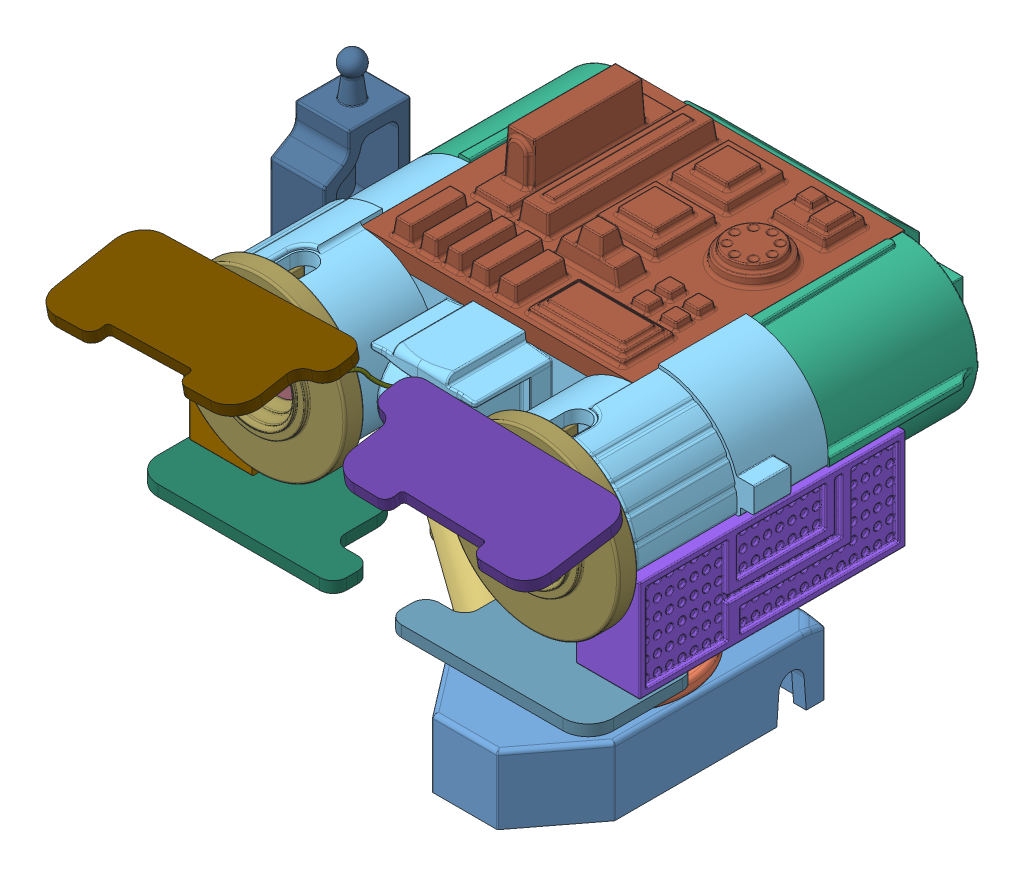
SolidWorks assembly Head, configuration Painted. Lengths in mm.
Overall size (59.38 58.47 64.88).
20 component instances, 18 part files, 63 mates.
Components (placement in the parent):
- Neck Block-1: Neck Block [Default] at origin size (19.8 8.1 32.9)
- Neck Column-1: Neck Column [Default] at (0 8.1 0) size (19.3 30.7 19.3)
- Neck Cylinders-1: Neck Cylinders [Default] at (0 9.78 6.15) size (41.82 28.67 7.85)
- Washer Head Thread-Forming Screw 2.6mm x 6mm-1: Washer Head Thread-Forming Screw 2.6mm x 6mm [Default] at (0 11.65 0) x (-0.707107 0 -0.707107) z (-0.707107 0 0.707107) size (7.8 7.44 7.8)
- Head (Front)-1: Head (Front) [Default] at (0 40.98 0) size (53.5 23.44 24.2)
- Head (Rear)-1: Head (Rear) [Default] at (0 40.98 0) size (51.98 22.63 26)
- Cheese Head Thread-Forming Screw 2.8mm x 8mm-1: Cheese Head Thread-Forming Screw 2.8mm x 8mm [Default] at (0 40.98 3.65) x (0.707107 -0.707107 0) z (0.707107 0.707107 0) size (5.45 9.97 5.45)
- Cheek (Left)-1: Cheek (Left) [Default] at (16.25 40.98 23) size (7.5 12 31.6)
- Cheek (Right)-1: Cheek (Right) [Default] at (-16.25 40.98 23) size (7.5 12 31.6)
- Whip Antenna-1: Whip Antenna [Default] at (-26.586 40.0668 10.4) size (6.56 18.4 10.28)
- Head Detail Plate-1: Head Detail Plate [Default] at (0 47.98 -2.935) size (32.69 7.75 31.87)
- Eye-3: Eye [Default] at (-16.25 40.98 23) size (20.5 20.5 7.96)
- Eye-4: Eye [Default] at (16.25 40.98 23) size (20.5 20.5 7.96)
- Lens-1: Lens [Painted] at (-16.25 40.98 23) size (10.8 10.8 0.8)
- Lens-2: Lens [Painted] at (16.25 40.98 23) size (10.8 10.8 0.8)
- Lower Eyeflap (Left)-1: Lower Eyeflap (Left) [Default] at (3.25 26.4828 29.4) size (23.8 1.32 12.82)
- Lower Eyeflap (Right)-1: Lower Eyeflap (Right) [Default] at (-3.25 26.4828 29.4) size (23.8 1.32 12.82)
- Eyeflap Wire-1: Eyeflap Wire [Default] at (0 46.2834 36.3285) x (1 0 0) z (0 0.173648 0.984808) size (22.36 3.31 16.37)
- Upper Eyeflap (Left)-1: Upper Eyeflap (Left) [Default] at (2.6277 49.0084 30.8173) x (0.99978 -0.019812 0.006846) z (-0.010094 -0.168795 0.985599) size (26.82 1.32 12.82)
- Upper Eyeflap (Right)-1: Upper Eyeflap (Right) [Default] at (-2.6331 49.0082 30.8174) x (0.999778 0.019901 -0.006876) z (0.010139 -0.168839 0.985592) size (26.82 1.32 12.82)
Mates (geometry in assembly coordinates):
- ROTATION LOCK: coincident aligned: plane of Neck Column-1 through (0 8.1 0) normal (0 0 1); plane of assembly through (0 0 0) normal (0 0 1)
- Coincident1: coincident: plane of Neck Block-1 through (0 0 0) normal (0 0 1); plane of assembly through (0 0 0) normal (0 0 1)
- Coincident2: coincident: plane of Neck Block-1 through (0 0 0) normal (0 1 0); plane of assembly through (0 0 0) normal (0 1 0)
- Coincident3: coincident aligned: plane of Neck Block-1 through (0 0 0) normal (1 0 0); plane of assembly through (0 0 0) normal (1 0 0)
- Concentric1: concentric anti-aligned: cylinder of Neck Block-1 through (0 8.1 0) axis (0 -1 0) radius 3; cylinder of Neck Column-1 through (0 5.85 0) axis (0 1 0) radius 2.885
- Coincident4: coincident anti-aligned: plane of Neck Block-1 through (0 8.1 0) normal (0 1 0); plane of Neck Column-1 through (0 8.1 0) normal (0 -1 0)
- Coincident12: coincident anti-aligned: plane of Neck Column-1 through (0 9.78 0) normal (0 1 0); plane of Neck Cylinders-1 through (0 9.78 6.15) normal (0 -1 0)
- Coincident13: coincident aligned: plane of Neck Column-1 through (0 8.1 0) normal (1 0 0); plane of Neck Cylinders-1 through (0 9.78 6.15) normal (1 0 0)
- Coincident14: coincident anti-aligned: plane of Neck Column-1 through (0 8.1 3.825) normal (0 0 1); plane of Neck Cylinders-1 through (0 10.78 3.825) normal (0 0 -1)
- Coincident6: coincident anti-aligned: plane of Head (Front)-1 through (0 40.0668 10.4) normal (0 1 0); plane of Whip Antenna-1 through (-23.306 40.0668 0.12) normal (0 -1 0)
- Coincident7: coincident anti-aligned: plane of Head (Front)-1 through (0 40.98 10.4) normal (0 0 -1); plane of Whip Antenna-1 through (-23.306 40.0668 10.4) normal (0 0 1)
- Coincident8: coincident anti-aligned: plane of Head (Front)-1 through (-23.306 40.98 10.4) normal (-1 0 0); plane of Whip Antenna-1 through (-23.306 40.0668 10.4) normal (1 0 0)
- Coincident16: coincident anti-aligned: plane of Head (Front)-1 through (-10.5931 47.98 -36.225) normal (0 1 0); plane of Head Detail Plate-1 through (0 47.98 -2.935) normal (0 -1 0)
- Coincident17: coincident anti-aligned: plane of Head (Front)-1 through (-16.25 40.98 13) normal (0 0 -1); plane of Head Detail Plate-1 through (-16.345 50.01 13) normal (0 0 1)
- Width1: width aligned: plane of Head Detail Plate-1 through (-16.345 50.01 13) normal (-1 0 0); plane of Head Detail Plate-1 through (16.345 50.01 13) normal (1 0 0); plane of Head (Front)-1 through (16.4 49.98 45.8609) normal (-1 0 0); plane of Head (Front)-1 through (-16.4 49.9787 37.0587) normal (1 0 0)
- Concentric9: concentric aligned: cylinder of Neck Column-1 through (0 27.55 0) axis (0 -1 0) radius 2.875; cylinder of Head (Front)-1 through (0 30.55 0) axis (0 -1 0) radius 3
- Parallel4: parallel aligned: plane of Neck Column-1 through (-4.9 19.43 4.9) normal (0 0 1); plane of Head (Front)-1 through (-16.25 40.98 13) normal (0 0 1)
- Concentric10: concentric aligned: cylinder of Eye-3 through (-16.25 40.98 18.2) axis (0 0 1) radius 6.02; cylinder of Lens-1 through (-16.25 40.98 22.2) axis (0 0 1) radius 5.4
- Concentric11: concentric aligned: cylinder of Head (Front)-1 through (-16.25 40.98 14) axis (0 0 1) radius 7.5; cylinder of Eye-3 through (-16.25 40.98 18.2) axis (0 0 1) radius 7.25
- Coincident19: coincident anti-aligned: plane of Head (Front)-1 through (-16.25 40.98 23) normal (0 0 1); plane of Eye-3 through (-16.25 40.98 23) normal (0 0 -1)
- Concentric12: concentric aligned: cylinder of Eye-4 through (16.25 40.98 18.2) axis (0 0 1) radius 6.02; cylinder of Lens-2 through (16.25 40.98 22.2) axis (0 0 1) radius 5.4
- Concentric13: concentric aligned: cylinder of Head (Front)-1 through (16.25 40.98 14) axis (0 0 1) radius 7.5; cylinder of Eye-4 through (16.25 40.98 18.2) axis (0 0 1) radius 7.25
- Coincident21: coincident anti-aligned: plane of Head (Front)-1 through (16.25 40.98 23) normal (0 0 1); plane of Eye-4 through (16.25 40.98 23) normal (0 0 -1)
- Coincident22: coincident aligned: plane of Head (Front)-1 through (0 40.98 0) normal (0 1 0); plane of Eye-3 through (-16.25 40.98 23) normal (0 1 0)
- Coincident23: coincident aligned: plane of Head (Front)-1 through (0 40.98 0) normal (0 1 0); plane of Eye-4 through (16.25 40.98 23) normal (0 1 0)
- Coincident24: coincident aligned: plane of Head (Front)-1 through (0 40.98 0) normal (0 1 0); plane of Lens-1 through (-16.25 40.98 23) normal (0 1 0)
- Coincident25: coincident aligned: plane of Head (Front)-1 through (0 40.98 0) normal (0 1 0); plane of Lens-2 through (16.25 40.98 23) normal (0 1 0)
- Coincident26: coincident anti-aligned: plane of Head (Front)-1 through (-16.25 40.98 0) normal (0 0 -1); plane of Head (Rear)-1 through (0 40.98 0) normal (0 0 1)
- Coincident27: coincident aligned: plane of Head (Front)-1 through (-10.5931 47.98 -36.225) normal (0 1 0); plane of Head (Rear)-1 through (-16.4 47.98 -18.7) normal (0 1 0)
- Concentric14: concentric anti-aligned: cylinder of Head (Front)-1 through (16.25 40.98 23) axis (0 0 -1) radius 9; cylinder of Head (Rear)-1 through (16.25 40.98 -18.7) axis (0 0 1) radius 9
- Coincident28: coincident anti-aligned: plane of Neck Column-1 through (0 27.55 0) normal (0 1 0); plane of Head (Front)-1 through (-9.73 27.55 14.5) normal (0 -1 0)
- Coincident30: coincident anti-aligned: plane of Eye-4 through (16.25 40.98 23) normal (0 0 -1); plane of Cheek (Left)-1 through (16.25 40.98 23) normal (0 0 1)
- Parallel5: parallel aligned: plane of Head (Rear)-1 through (-16.4 50.33 -18.7) normal (0 1 0); plane of Cheek (Left)-1 through (25.1727 29.8028 21.5) normal (0 1 0)
- Concentric16: concentric aligned: cylinder of Head (Rear)-1 through (16.25 40.98 -18.7) axis (0 0 1) radius 9; cylinder of Cheek (Left)-1 through (16.25 40.98 -8.6) axis (0 0 1) radius 9
- Concentric18: concentric aligned: cylinder of Neck Column-1 through (0 5.85 0) axis (0 -1 0) radius 0.8; cylinder of Washer Head Thread-Forming Screw 2.6mm x 6mm-1 through (0 4.25 0) axis (0 -1 0) radius 1.3
- Coincident31: coincident anti-aligned: plane of Neck Column-1 through (0 5.85 0) normal (0 -1 0); plane of Washer Head Thread-Forming Screw 2.6mm x 6mm-1 through (0.9192 5.85 0.9192) normal (0 1 0)
- Angle3: planar angle = 0.785398 rad aligned: plane of Washer Head Thread-Forming Screw 2.6mm x 6mm-1 through (0 11.65 0) normal (-0.707107 0 0.707107); plane of Neck Column-1 through (0 8.1 0) normal (0 0 1)
- Concentric19: concentric aligned: cylinder of Head (Front)-1 through (0 40.98 -1.2) axis (0 0 -1) radius 0.9; cylinder of Cheese Head Thread-Forming Screw 2.8mm x 8mm-1 through (0 40.98 -6.25) axis (0 0 -1) radius 1.4
- Coincident32: coincident anti-aligned: plane of Head (Rear)-1 through (12.075 40.98 -4.05) normal (0 0 -1); plane of Cheese Head Thread-Forming Screw 2.8mm x 8mm-1 through (-0.9899 41.9699 -4.05) normal (0 0 1)
- Angle4: planar angle = 0.785398 rad aligned: plane of Cheese Head Thread-Forming Screw 2.8mm x 8mm-1 through (0 40.98 3.65) normal (0.707107 0.707107 0); plane of Head (Front)-1 through (0 40.98 0) normal (1 0 0)
- Coincident34: coincident anti-aligned: plane of Cheek (Right)-1 through (-16.25 40.98 23) normal (0 0 1); plane of Eye-3 through (-16.25 40.98 23) normal (0 0 -1)
- Parallel6: parallel anti-aligned: plane of Head (Rear)-1 through (-16.4 50.33 -18.7) normal (0 1 0); plane of Cheek (Right)-1 through (-19.2727 27.8028 -8.6) normal (0 -1 0)
- Concentric20: concentric aligned: cylinder of Head (Rear)-1 through (-16.25 40.98 -18.7) axis (0 0 1) radius 9; cylinder of Cheek (Right)-1 through (-16.25 40.98 -8.6) axis (0 0 1) radius 9
- Coincident38: coincident anti-aligned: plane of Cheek (Left)-1 through (19.2727 27.8028 -8.6) normal (0 -1 0); plane of Lower Eyeflap (Left)-1 through (3.25 27.8028 29.4) normal (0 1 0)
- Coincident39: coincident anti-aligned: plane of Cheek (Right)-1 through (-19.2727 27.8028 -8.6) normal (0 -1 0); plane of Lower Eyeflap (Right)-1 through (-3.25 27.8028 29.4) normal (0 1 0)
- Coincident40: coincident aligned: plane of Lower Eyeflap (Left)-1 through (3.25 27.8028 29.4) normal (0 0 1); plane of Lower Eyeflap (Right)-1 through (-3.25 27.8028 29.4) normal (0 0 1)
- Distance1: distance = 6.4 mm aligned: plane of Lower Eyeflap (Right)-1 through (-3.25 27.8028 29.4) normal (0 0 1); plane of Cheek (Right)-1 through (-16.25 40.98 23) normal (0 0 1)
- Distance2: distance = 6.5 mm anti-aligned: plane of Lower Eyeflap (Left)-1 through (3.25 27.8028 29.4) normal (-1 0 0); plane of Lower Eyeflap (Right)-1 through (-3.25 27.8028 29.4) normal (1 0 0)
- Coincident42: coincident aligned: plane of Eyeflap Wire-1; plane of Head (Front)-1 through (0 40.98 0) normal (1 0 0)
- Angle5: planar angle = 0.174533 rad aligned: plane of Eyeflap Wire-1 through (0 46.2834 36.3285) normal (0 0.984808 -0.173648); plane of assembly through (0 0 0) normal (0 1 0)
- Tangent1: tangent anti-aligned: cylinder of Eyeflap Wire-1 through (3.539 49.2131 28.3406) axis (0.95126 -0.069258 0.300514) radius 0.2; plane of Upper Eyeflap (Left)-1 through (2.6277 49.0084 30.8173) normal (-0.018372 -0.985452 -0.168958)
- Tangent2: tangent anti-aligned: cylinder of Eyeflap Wire-1 through (10.9778 48.5469 31.4175) axis (-0.010094 -0.168795 0.985599) radius 0.2; plane of Upper Eyeflap (Left)-1 through (2.6277 49.0084 30.8173) normal (-0.018372 -0.985452 -0.168958)
- Distance3: distance = 1 mm aligned: plane of Upper Eyeflap (Left)-1 through (12.4107 49.1272 36.8733) normal (-0.010094 -0.168795 0.985599); plane of Eyeflap Wire-1 through (10.9347 47.827 35.6209) normal (-0.010094 -0.168795 0.985599)
- Tangent5: tangent: plane of Head (Front)-1 through (-2.25 44.98 19.62) normal (0 0 1); face of Eyeflap Wire-1
- Tangent9: tangent anti-aligned: cylinder of Eyeflap Wire-1 through (-10.2858 48.7211 30.4722) axis (0.951244 0.069356 -0.30054) radius 0.2; plane of Upper Eyeflap (Right)-1 through (-2.6331 49.0082 30.8174) normal (0.018454 -0.985443 -0.169003)
- Tangent7: tangent anti-aligned: cylinder of Eyeflap Wire-1 through (-10.9777 48.546 31.4178) axis (0.010139 -0.168839 0.985592) radius 0.2; plane of Upper Eyeflap (Right)-1 through (-2.6331 49.0082 30.8174) normal (0.018454 -0.985443 -0.169003)
- Distance4: distance = 1 mm aligned: plane of Upper Eyeflap (Right)-1 through (-12.416 49.1258 36.8737) normal (0.010139 -0.168839 0.985592); plane of Eyeflap Wire-1 through (-10.9344 47.8259 35.6211) normal (0.010139 -0.168839 0.985592)
- Tangent10: tangent: plane of Head (Front)-1 through (-2.25 44.98 21.8683) normal (0 1 0); face of Eyeflap Wire-1
- Coincident43: coincident anti-aligned: plane of Eye-3 through (-16.25 40.98 23) normal (0 0 -1); plane of Lens-1 through (-16.25 40.98 23) normal (0 0 1)
- Coincident44: coincident anti-aligned: plane of Eye-4 through (16.25 40.98 23) normal (0 0 -1); plane of Lens-2 through (16.25 40.98 23) normal (0 0 1)
- Symmetric1: symmetric aligned: plane of Head (Front)-1 through (0 40.98 0) normal (1 0 0); plane of Lower Eyeflap (Left)-1 through (3.25 27.8028 29.4) normal (-1 0 0); plane of Lower Eyeflap (Right)-1 through (-3.25 27.8028 29.4) normal (1 0 0)
- Distance7: distance = 1.1 mm: line of Lower Eyeflap (Left)-1 through (27.05 27.8028 26.4) axis (0 0 -1); line of Upper Eyeflap (Left)-1 through (29.4139 48.9052 36.3195) axis (0.010094 0.168795 -0.985599)
- Distance8: distance = 1.1 mm: line of Upper Eyeflap (Right)-1 through (-29.4191 48.9023 36.3204) axis (-0.010139 0.168839 -0.985592); line of Lower Eyeflap (Right)-1 through (-27.05 27.8028 26.4) axis (0 0 -1)
